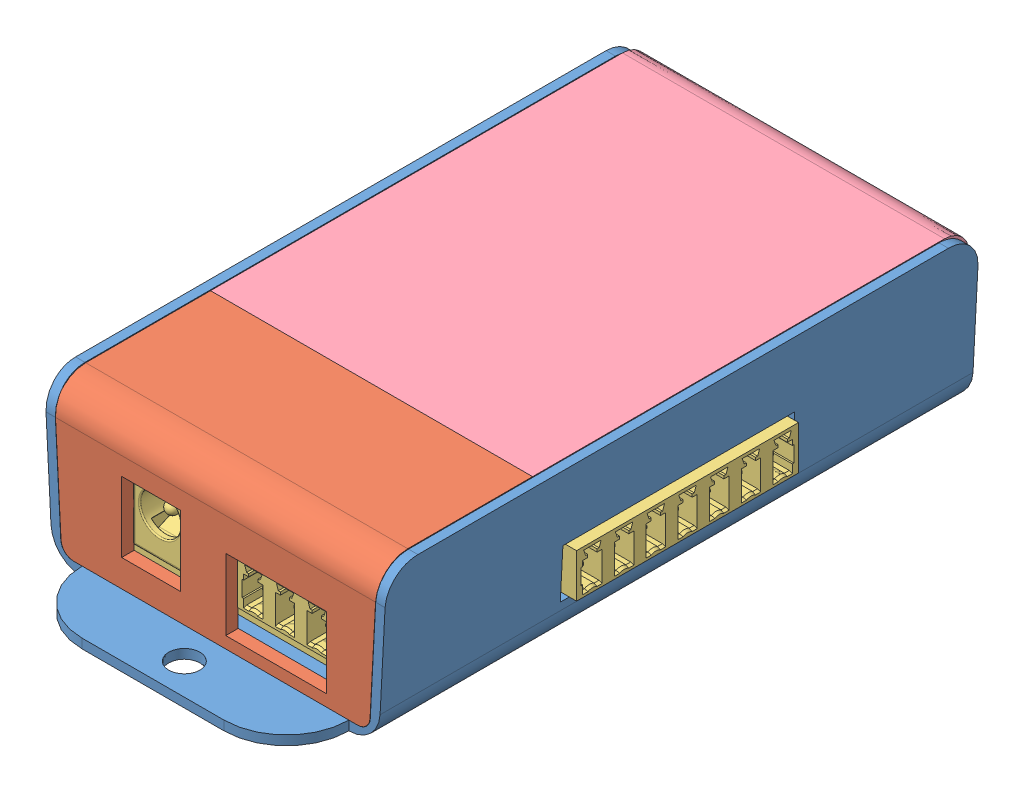
SolidWorks assembly Assembly, configuration Default. Lengths in mm.
Overall size (55.61 25 115).
5 component instances, 5 part files, 13 mates.
Components (placement in the parent):
- Bottom-1: Bottom [Default] at origin size (54.85 25 115)
- top-1: top [Default] at (0 1.5 47.5) size (51.6 23.5 95)
- PCB1-2: PCB1 [Default] at (-97.96 6.5908 139.76) x (1 0 0) z (0 1 0) size (52.58 90.2 14.6)
- TOP COVER-1: TOP COVER [Default] at (-25.8 1.5 47.5029) x (0 0 -1) z (1 0 0) size (72 21.61 51.6) (hidden)
- sim7000g-2: sim7000g [Default] at (-17.8 17.2408 35.5) x (0 0 1) z (0 1 0) size (38 37 13.34)
Mates (geometry in assembly coordinates):
- Coincident1: coordinate: point of Bottom-1; point of assembly
- Coincident2: coincident anti-aligned: plane of Bottom-1 through (17 5 29.5) normal (0 1 0); plane of PCB1-2 through (0 5 50.4369) normal (0 -1 0)
- Concentric1: concentric aligned: cylinder of Bottom-1 through (18.5 11.4 21.5) axis (0 -1 0) radius 2.5; cylinder of PCB1-2 through (18.5 5 21.5) axis (0 -1 0) radius 2.5
- Parallel1: parallel aligned: plane of Bottom-1 through (0 0 95) normal (0 0 1); plane of PCB1-2 through (23.5 5 92.7) normal (0 0 1)
- Coincident3: coincident aligned: plane of Bottom-1 through (24.9216 25 95) normal (0 1 0); plane of top-1 through (-25.8 25 0) normal (0 1 0)
- Coincident4: coincident anti-aligned: plane of top-1 through (-30.2 20 1) normal (0 0 -1); plane of TOP COVER-1 through (25.8 20 1) normal (0 0 1)
- Coincident5: coincident aligned: plane of top-1 through (-25.8 25 0) normal (0 1 0); plane of TOP COVER-1 through (25.8 25 0) normal (0 1 0)
- Coincident6: coincident anti-aligned: line of top-1 through (-25.8 23.9986 70) axis (0 0 -1); line of TOP COVER-1 through (-25.8 23.9986 4.8983) axis (0 0 1)
- Concentric3: concentric aligned: cylinder of Bottom-1 through (-18.5 -3.6 73.5) axis (0 1 0) radius 1.65; cylinder of top-1 through (-18.5 14 73.5) axis (0 1 0) radius 2.3
- Concentric4: concentric aligned: cylinder of Bottom-1 through (18.5 -3.6 21.5) axis (0 1 0) radius 1.65; cylinder of top-1 through (18.5 14 21.5) axis (0 1 0) radius 2.3
- Distance1: distance = 8 mm anti-aligned: plane of PCB1-2 through (0 6.5908 50.4369) normal (0 1 0); plane of sim7000g-2 through (-10.85 14.5908 42.7) normal (0 -1 0)
- Distance2: distance = 5 mm anti-aligned: plane of top-1 through (-22.8 -32.0014 70) normal (1 0 0); plane of sim7000g-2 through (-17.8 17.2408 35.5) normal (-1 0 0)
- Distance3: distance = 33.5 mm anti-aligned: plane of top-1 through (-25.8 23 2) normal (0 0 1); plane of sim7000g-2 through (19.2 17.2408 35.5) normal (0 0 -1)
